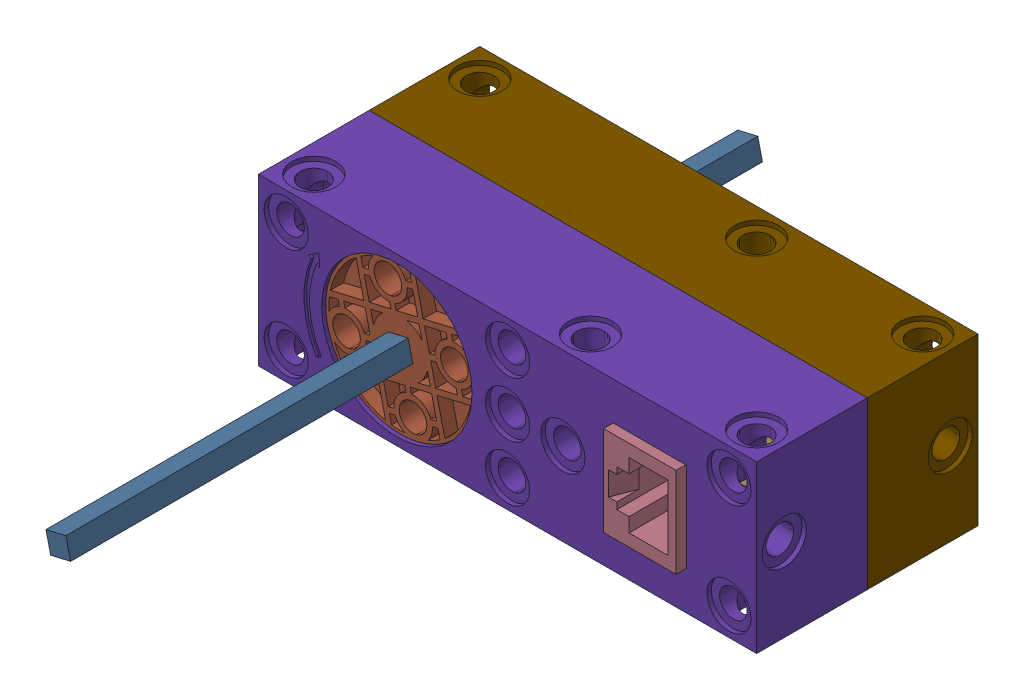
SolidWorks assembly 玩具装配体-修改V1版_arrow, configuration Default. Lengths in mm.
Overall size (100.85 33.6 125).
27 component instances, 18 part files, 0 mates.
Components (placement in the parent):
- 玩具装配体-修改V1版(2)^玩具装配体-修改V1版_arrow-1: 玩具装配体-修改V1版(2)^玩具装配体-修改V1版_arrow [Default] at origin size (100.85 33.6 125) (virtual)
  - ____________ __^玩具装配体-修改V1版(2)_玩具装配体-修改V1版_arrow-1: ____________ __^玩具装配体-修改V1版(2)_玩具装配体-修改V1版_arrow [Default] at (-20.5104 -47.3194 -73.272) size (78.96 33.52 125) (virtual)
    - ________^____________ ___玩具装配体-修改V1版(2)_玩具装配体-修改V1版_arrow-1: ________^____________ ___玩具装配体-修改V1版(2)_玩具装配体-修改V1版_arrow [Default] at (-3.235 23.1684 17.3007) size (77.01 26.03 28.01) (virtual)
      - ________-1^_____________________ ___玩具装配体-修改V1版(2)_玩具装配体-修改V1版_arrow-1: ________-1^_____________________ ___玩具装配体-修改V1版(2)_玩具装配体-修改V1版_arrow [Default] at (78.0405 10.9538 66.5002) x (0 1 0) z (-1 0 0) size (20.4 27.91 40.6) (virtual)
        - 130____^________-1______________________ ___玩具装配体-修改V1版(2)_玩具装配体-修改V1版_arrow-1: 130____^________-1______________________ ___玩具装配体-修改V1版(2)_玩具装配体-修改V1版_arrow [Default] at (13.1972 32.2289 22.095) size (20.4 15.42 40.6) (virtual)
        - _________GearTrax^________-1______________________ ___玩具装配体-修改V1版(2)_玩具装配体-修改V1版_arrow-1: _________GearTrax^________-1______________________ ___玩具装配体-修改V1版(2)_玩具装配体-修改V1版_arrow [Default] at (13.1972 32.2289 59.5205) size (5.14 5.15 2.51) (virtual)
        - ______1^________-1______________________ ___玩具装配体-修改V1版(2)_玩具装配体-修改V1版_arrow-1: ______1^________-1______________________ ___玩具装配体-修改V1版(2)_玩具装配体-修改V1版_arrow [Default] at (13.1972 32.2289 21.345) x (-1 0 0) z (0 0 -1) size (19.6 27.5 1.5) (virtual)
      - ____^_____________________ ___玩具装配体-修改V1版(2)_玩具装配体-修改V1版_arrow-1: ____^_____________________ ___玩具装配体-修改V1版(2)_玩具装配体-修改V1版_arrow [Default] at (-11.0546 37.151 26.4713) size (42.03 26.03 17.01) (virtual)
      - ____-0^_____________________ ___玩具装配体-修改V1版(2)_玩具装配体-修改V1版_arrow-1: ____-0^_____________________ ___玩具装配体-修改V1版(2)_玩具装配体-修改V1版_arrow [Default] at (19.3454 24.151 27.4713) x (0.849881 -0.526974 0) z (0 0 1) size (2 2 17.3) (virtual)
    - Z38M0.6__18.9__^____________ ___玩具装配体-修改V1版(2)_玩具装配体-修改V1版_arrow-1: Z38M0.6__18.9__^____________ ___玩具装配体-修改V1版(2)_玩具装配体-修改V1版_arrow [Default] at (-3903.5586 351.9955 56.972) x (-0.227574 0.973761 0) z (0 0 1) size (23.9 23.96 36.6) (virtual)
    - ____-1^____________ ___玩具装配体-修改V1版(2)_玩具装配体-修改V1版_arrow-1: ____-1^____________ ___玩具装配体-修改V1版(2)_玩具装配体-修改V1版_arrow [Default] at (-14.2896 34.3194 62.772) x (1 0 0) z (0 0 -1) size (42 26 18.5) (virtual)
    - ________-2^____________ ___玩具装配体-修改V1版(2)_玩具装配体-修改V1版_arrow-1: ________-2^____________ ___玩具装配体-修改V1版(2)_玩具装配体-修改V1版_arrow [Default] at (-11.2896 57.3194 61.772) x (0.500769 -0.865581 0) z (0 0 -1) size (3.8 3.8 14.01) (virtual)
    - ________-2^____________ ___玩具装配体-修改V1版(2)_玩具装配体-修改V1版_arrow-2: ________-2^____________ ___玩具装配体-修改V1版(2)_玩具装配体-修改V1版_arrow [Default] at (24.7104 57.3194 61.772) x (0.500769 -0.865581 0) z (0 0 -1) size (3.8 3.8 14.01) (virtual)
    - ________-2^____________ ___玩具装配体-修改V1版(2)_玩具装配体-修改V1版_arrow-3: ________-2^____________ ___玩具装配体-修改V1版(2)_玩具装配体-修改V1版_arrow [Default] at (24.7104 37.3194 61.772) x (0.500769 -0.865581 0) z (0 0 -1) size (3.8 3.8 14.01) (virtual)
    - ________-2^____________ ___玩具装配体-修改V1版(2)_玩具装配体-修改V1版_arrow-4: ________-2^____________ ___玩具装配体-修改V1版(2)_玩具装配体-修改V1版_arrow [Default] at (-11.2896 37.3194 61.772) x (0.500769 -0.865581 0) z (0 0 -1) size (3.8 3.8 14.01) (virtual)
    - ________-3^____________ ___玩具装配体-修改V1版(2)_玩具装配体-修改V1版_arrow-1: ________-3^____________ ___玩具装配体-修改V1版(2)_玩具装配体-修改V1版_arrow [Default] at (31.2104 53.2694 51.572) x (0 -0.340814 0.940131) z (-1 0 0) size (3.6 3.6 6.21) (virtual)
    - ________-3^____________ ___玩具装配体-修改V1版(2)_玩具装配体-修改V1版_arrow-2: ________-3^____________ ___玩具装配体-修改V1版(2)_玩具装配体-修改V1版_arrow [Default] at (31.2104 40.8694 51.572) x (0 -0.063636 0.997973) z (-1 0 0) size (3.6 3.6 6.21) (virtual)
    - ______^____________ ___玩具装配体-修改V1版(2)_玩具装配体-修改V1版_arrow-1: ______^____________ ___玩具装配体-修改V1版(2)_玩具装配体-修改V1版_arrow [Default] at (0.5104 47.3194 71.9404) x (-0.227574 0.973761 0) z (0 0 1) size (3.7 3.7 125) (virtual)
    - ____-4^____________ ___玩具装配体-修改V1版(2)_玩具装配体-修改V1版_arrow-1: ____-4^____________ ___玩具装配体-修改V1版(2)_玩具装配体-修改V1版_arrow [Default] at (0.5104 47.3194 72.622) x (0 0 -1) z (0.973761 0.227574 0) size (8.4 27.9 27.9) (virtual)
    - ____-4^____________ ___玩具装配体-修改V1版(2)_玩具装配体-修改V1版_arrow-2: ____-4^____________ ___玩具装配体-修改V1版(2)_玩具装配体-修改V1版_arrow [Default] at (0.5104 47.3194 33.922) x (0 0 1) z (-1 0 0) size (8.4 27.9 27.9) (virtual)
    - ____-5^____________ ___玩具装配体-修改V1版(2)_玩具装配体-修改V1版_arrow-1: ____-5^____________ ___玩具装配体-修改V1版(2)_玩具装配体-修改V1版_arrow [Default] at (59.6947 47.3194 51.572) x (0 0.059635 0.99822) z (-1 0 0) size (14 14 5.5) (virtual)
    - 56-L-8P8C^____________ ___玩具装配体-修改V1版(2)_玩具装配体-修改V1版_arrow-1: 56-L-8P8C^____________ ___玩具装配体-修改V1版(2)_玩具装配体-修改V1版_arrow [Default] at (46.1604 47.3194 67.147) x (0 1 0) z (0 0 -1) size (16.26 16.5 15.75) (virtual)
    - Z22M0.6 Z38 M0.6^____________ ___玩具装配体-修改V1版(2)_玩具装配体-修改V1版_arrow-1: Z22M0.6 Z38 M0.6^____________ ___玩具装配体-修改V1版(2)_玩具装配体-修改V1版_arrow [Default] at (4055.0964 -742.0967 52.772) x (0.498442 0.866923 0) z (0 0 -1) size (23.9 23.96 6) (virtual)
    - Z13M0.6__5.5__Z30M0.6^____________ ___玩具装配体-修改V1版(2)_玩具装配体-修改V1版_arrow-1: Z13M0.6__5.5__Z30M0.6^____________ ___玩具装配体-修改V1版(2)_玩具装配体-修改V1版_arrow [Default] at (1788.7009 3696.9599 56.372) x (0.992497 -0.122272 0) z (0 0 1) size (18.53 18.6 6) (virtual)
    - ________A_GearTrax^____________ ___玩具装配体-修改V1版(2)_玩具装配体-修改V1版_arrow-1: ________A_GearTrax^____________ ___玩具装配体-修改V1版(2)_玩具装配体-修改V1版_arrow [Default] at (16.1104 47.3194 51.2492) x (0.992424 -0.122859 0) z (0 0 1) size (19.01 19.02 5.9) (virtual)
  - ____1A-1: ____1A [Default] x (1 0 0) z (0 0 -1) size (100.85 33.6 20)
  - ____2A-1: ____2A [Default] at (0 0 -40) size (90 30 22)
